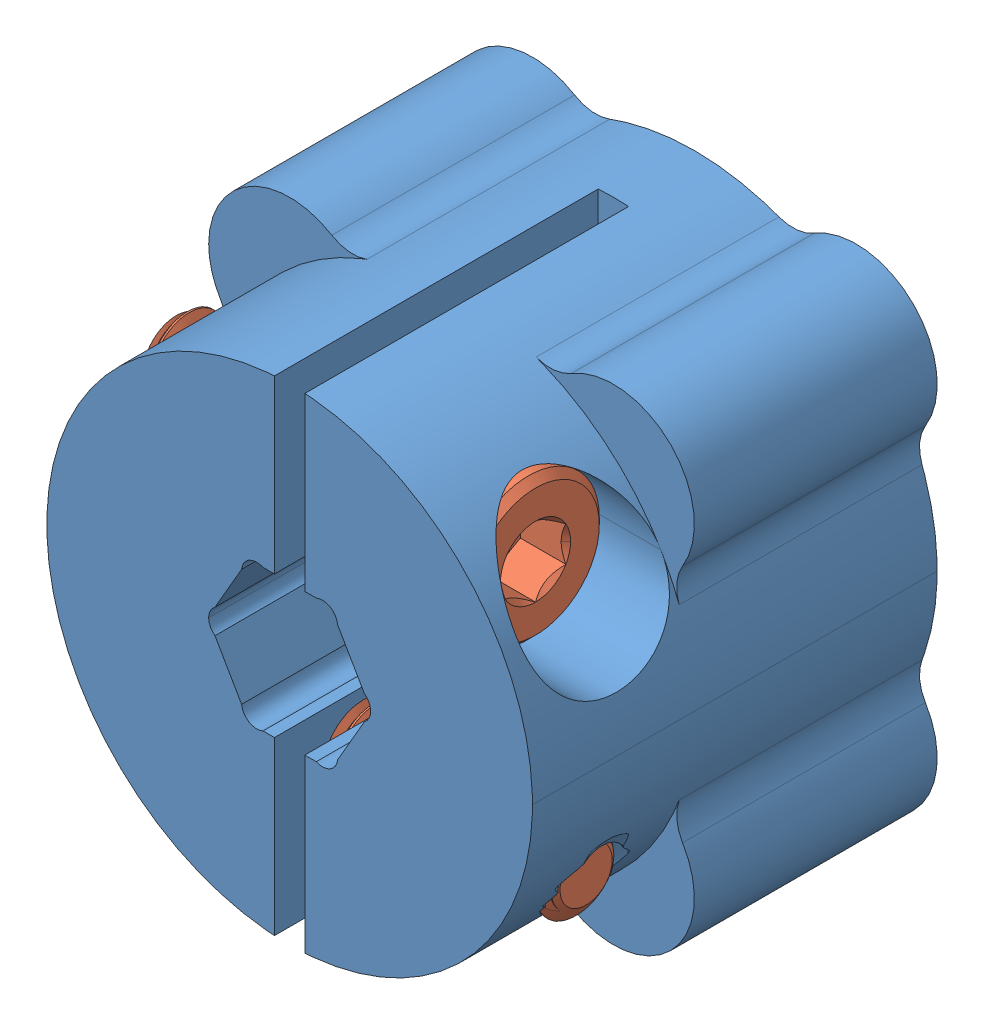
SolidWorks assembly 1310-0016-4008 assembly, configuration Default. Lengths in mm.
Overall size (24 24 22).
4 component instances, 2 part files, 0 mates.
Components (placement in the parent):
- 1310-0016-4008 assembly.STEP-1: 1310-0016-4008 assembly.STEP [Default] at origin size (24 24 22)
  - 1310-0016-4008.STEP-1: 1310-0016-4008.STEP [Default] at (-14.0123 7.4584 -7.173) size (24 24 22)
  - 2800-0004-0014_90128A207.STEP-1: 2800-0004-0014_90128A207.STEP [Default] at (-3.7623 1.38 8.427) x (0 0 -1) z (1 0 0) size (7 7 18.01)
  - 2800-0004-0014_90128A207.STEP-2: 2800-0004-0014_90128A207.STEP [Default] at (-24.2623 13.5369 8.427) x (0 0 1) z (-1 0 0) size (7 7 18.01)
